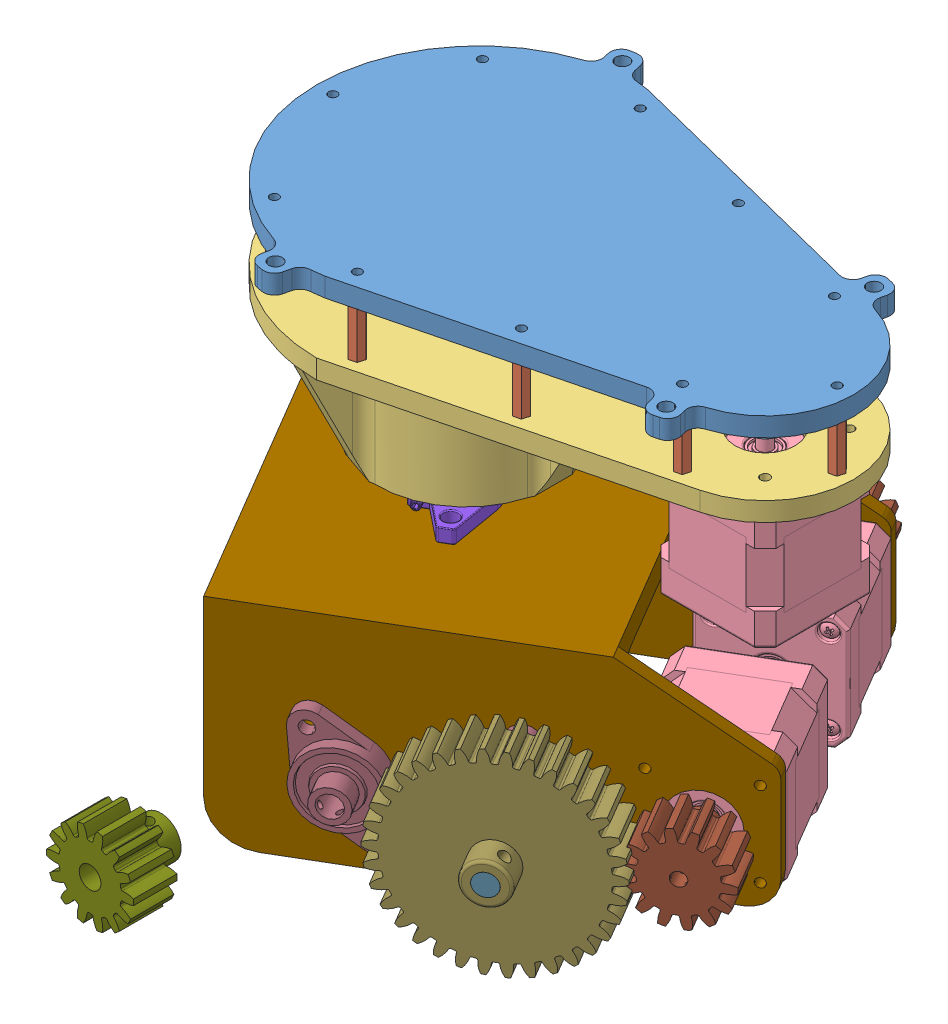
SolidWorks assembly Assembly, configuration Default. Lengths in mm.
Overall size (223.52 202.91 241.25).
33 component instances, 16 part files, 73 mates.
Components (placement in the parent):
- base1-2: base1 [Varsayılan] at (61.0141 100.5381 159.3571) size (197.5 7 137.85)
- tru_dong_20mm-1: tru_dong_20mm [Default] at (-33.0715 80.5381 158.3482) x (-1 0 0) z (0 1 0) size (5.26 5.22 20)
- tru_dong_20mm-2: tru_dong_20mm [Default] at (-16.7501 80.5381 119.6659) x (-1 0 0) z (0 1 0) size (5.26 5.22 20)
- tru_dong_20mm-3: tru_dong_20mm [Default] at (123.4514 80.5381 130.3946) x (-1 0 0) z (0 1 0) size (5.26 5.22 20)
- tru_dong_20mm-4: tru_dong_20mm [Default] at (27.9599 80.5381 210.3868) x (-1 0 0) z (0 1 0) size (5.26 5.22 20)
- tru_dong_20mm-5: tru_dong_20mm [Default] at (76.1904 80.5381 118.4744) x (-1 0 0) z (0 1 0) size (5.26 5.22 20)
- tru_dong_20mm-6: tru_dong_20mm [Default] at (-11.1111 80.5381 201.8162) x (-1 0 0) z (0 1 0) size (5.26 5.22 20)
- tru_dong_20mm-7: tru_dong_20mm [Default] at (152.4285 80.5381 158.3482) x (-1 0 0) z (0 1 0) size (5.26 5.22 20)
- tru_dong_20mm-8: tru_dong_20mm [Default] at (123.4514 80.5381 186.3018) x (-1 0 0) z (0 1 0) size (5.26 5.22 20)
- tru_dong_20mm-9: tru_dong_20mm [Default] at (27.9599 80.5381 106.3096) x (-1 0 0) z (0 1 0) size (5.26 5.22 20)
- tru_dong_20mm-10: tru_dong_20mm [Default] at (76.1904 80.5381 198.222) x (-1 0 0) z (0 1 0) size (5.26 5.22 20)
- base2-1: base2 [Varsayılan] at (55.9285 80.5381 158.3482) x (-1 0 0) z (0 0 1) size (197.5 57 120)
- NEMA 17-1: NEMA 17 [Default] at (121.3113 29.5381 168.7437) x (0 0 1) z (0 1 0) size (42.3 42.3 68)
- GT2_16T-1: GT2_16T [Default] at (125.9285 90.4881 158.3482) x (-0.780314 0 -0.625388) z (0 -1 0) size (13.6 13.6 15.5)
- GT2_80T_8mmSLDPRT-1: GT2_80T_8mmSLDPRT [Default] at (15.9285 83.5381 158.3482) x (0.428158 0 -0.903704) z (0 1 0) size (55 55 18)
- F608ZZ-1: F608ZZ [Défaut] at (15.9285 25.5381 158.3482) x (0.989487 0 0.144619) z (0 -1 0) size (25 25 7)
- SHF-8-1: SHF-8 [Default] at (15.9285 3.5381 158.3482) x (-0.508063 0 -0.86132) z (0.86132 0 -0.508063) size (43 10.01 24)
- base3-1: base3 [Varsayılan] at (15.9285 -5.4619 158.3482) x (0.508063 0 0.86132) z (-0.86132 0 0.508063) size (120 79 155)
- NEMA 17-2: NEMA 17 [Default] at (87.3379 -41.2437 103.4551) x (0.86132 0 -0.508063) z (-0.508063 0 -0.86132) size (42.3 42.3 68)
- NEMA 17-3: NEMA 17 [Default] at (85.5846 -56.2564 130.0315) x (0 -1 0) z (0.508063 0 0.86132) size (42.3 42.3 68)
- truc8_107mm-1: truc8_107mm [Default] at (15.9285 101.5381 158.3482) x (1 0 0) z (0 -1 0) size (8 8 107)
- banh_rang_1-2: banh_rang_1 [Varsayılan] at (123.0936 -45.8609 184.5328) x (-0.491421 0.821267 0.289873) z (-0.508063 0 -0.86132) size (32 32 26)
- banh_rang_1-3: banh_rang_1 [Varsayılan] at (44.8518 -45.8609 51.8896) x (0.859443 -0.065982 -0.506956) z (0.508063 0 0.86132) size (32 32 26)
- banh_rang_2-1: banh_rang_2 [Varsayılan] at (0.9682 -45.8609 71.97) x (0.433616 0.864035 -0.255775) z (0.508063 0 0.86132) size (72 72 26)
- KFL08-1: KFL08 [По умолчанию] at (12.1456 -45.8609 90.9191) x (-0.86132 0 0.508063) z (-0.508063 0 -0.86132) size (27 47.5 16)
- KFL08-2: KFL08 [По умолчанию] at (-29.1978 -45.8609 115.3061) x (-0.745925 -0.5 0.439996) z (-0.508063 0 -0.86132) size (27 47.5 16)
- KFL08-3: KFL08 [По умолчанию] at (73.1132 -45.8609 194.2774) x (0.86132 0 -0.508063) z (0.508063 0 0.86132) size (27 47.5 16)
- KFL08-4: KFL08 [По умолчанию] at (31.7698 -45.8609 218.6645) x (0.745925 0.5 -0.439996) z (0.508063 0 0.86132) size (27 47.5 16)
- banh_rang_2-2: banh_rang_2 [Varsayılan] at (84.2906 -45.8609 213.2265) x (-0.734353 0.522579 0.43317) z (-0.508063 0 -0.86132) size (72 72 26)
- truc8_200mm-1: truc8_200mm [Default] at (-8.177 -45.8609 56.4663) x (0.095955 -0.993775 -0.056601) z (0.508063 0 0.86132) size (8 8 200)
- banh_rang_3-1: banh_rang_3 [Varsayılan] at (-21.551 -45.8609 128.2697) x (0.813523 -0.32849 -0.47987) z (0.508063 0 0.86132) size (72 72 16)
- banh_rang_3-2: banh_rang_3 [Varsayılan] at (1.1002 -45.8609 166.6703) x (0.813523 -0.32849 -0.47987) z (0.508063 0 0.86132) size (72 72 16)
- banh_rang_4-1: banh_rang_4 [Varsayılan] at (-7.9995 -72.1728 264.7065) size (32 32 26)
Mates (geometry in assembly coordinates):
- Coincident1: coincident aligned: plane of tru_dong_20mm-1 through (-33.0715 80.5381 158.3482) normal (0 -1 0); plane of tru_dong_20mm-2 through (-16.7501 80.5381 119.6659) normal (0 -1 0)
- Coincident2: coincident aligned: plane of tru_dong_20mm-2 through (-16.7501 80.5381 119.6659) normal (0 -1 0); plane of tru_dong_20mm-3 through (123.4514 80.5381 130.3946) normal (0 -1 0)
- Coincident3: coincident aligned: plane of tru_dong_20mm-3 through (123.4514 80.5381 130.3946) normal (0 -1 0); plane of tru_dong_20mm-4 through (27.9599 80.5381 210.3868) normal (0 -1 0)
- Coincident4: coincident aligned: plane of tru_dong_20mm-4 through (27.9599 80.5381 210.3868) normal (0 -1 0); plane of tru_dong_20mm-5 through (76.1904 80.5381 118.4744) normal (0 -1 0)
- Coincident5: coincident aligned: plane of tru_dong_20mm-3 through (123.4514 80.5381 130.3946) normal (0 -1 0); plane of tru_dong_20mm-6 through (-11.1111 80.5381 201.8162) normal (0 -1 0)
- Coincident6: coincident aligned: plane of tru_dong_20mm-3 through (123.4514 80.5381 130.3946) normal (0 -1 0); plane of tru_dong_20mm-7 through (152.4285 80.5381 158.3482) normal (0 -1 0)
- Coincident7: coincident aligned: plane of tru_dong_20mm-3 through (123.4514 80.5381 130.3946) normal (0 -1 0); plane of tru_dong_20mm-9 through (27.9599 80.5381 106.3096) normal (0 -1 0)
- Coincident8: coincident aligned: plane of tru_dong_20mm-6 through (-11.1111 80.5381 201.8162) normal (0 -1 0); plane of tru_dong_20mm-8 through (123.4514 80.5381 186.3018) normal (0 -1 0)
- Coincident9: coincident aligned: plane of tru_dong_20mm-8 through (123.4514 80.5381 186.3018) normal (0 -1 0); plane of tru_dong_20mm-10 through (76.1904 80.5381 198.222) normal (0 -1 0)
- Coincident10: coincident anti-aligned: plane of base1-2 through (125.9285 100.5381 158.3482) normal (0 -1 0); plane of tru_dong_20mm-5 through (76.1904 100.5381 118.4744) normal (0 1 0)
- Concentric1: concentric aligned: cylinder of base1-2 through (76.1904 107.5381 118.4744) axis (0 -1 0) radius 1.6; cylinder of tru_dong_20mm-5 through (76.1904 100.5381 118.4744) axis (0 -1 0) radius 1.6
- Concentric2: concentric aligned: cylinder of base1-2 through (-16.7501 107.5381 119.6659) axis (0 -1 0) radius 1.6; cylinder of tru_dong_20mm-2 through (-16.7501 100.5381 119.6659) axis (0 -1 0) radius 1.6
- Concentric3: concentric aligned: cylinder of base1-2 through (-33.0715 107.5381 158.3482) axis (0 -1 0) radius 1.6; cylinder of tru_dong_20mm-1 through (-33.0715 100.5381 158.3482) axis (0 -1 0) radius 1.6
- Concentric4: concentric aligned: cylinder of base1-2 through (27.9599 107.5381 106.3096) axis (0 -1 0) radius 1.6; cylinder of tru_dong_20mm-9 through (27.9599 100.5381 106.3096) axis (0 -1 0) radius 1.6
- Concentric5: concentric aligned: cylinder of base1-2 through (123.4514 107.5381 130.3946) axis (0 -1 0) radius 1.6; cylinder of tru_dong_20mm-3 through (123.4514 100.5381 130.3946) axis (0 -1 0) radius 1.6
- Concentric6: concentric aligned: cylinder of base1-2 through (152.4285 107.5381 158.3482) axis (0 -1 0) radius 1.6; cylinder of tru_dong_20mm-7 through (152.4285 100.5381 158.3482) axis (0 -1 0) radius 1.6
- Coincident11: coincident anti-aligned: circle of base1-2; cylinder of tru_dong_20mm-8 through (123.4514 100.5381 186.3018) axis (0 -1 0) radius 1.6
- Concentric7: concentric aligned: cylinder of base1-2 through (76.1904 107.5381 198.222) axis (0 -1 0) radius 1.6; cylinder of tru_dong_20mm-10 through (76.1904 100.5381 198.222) axis (0 -1 0) radius 1.6
- Concentric8: concentric aligned: cylinder of base1-2 through (27.9599 107.5381 210.3868) axis (0 -1 0) radius 1.6; cylinder of tru_dong_20mm-4 through (27.9599 100.5381 210.3868) axis (0 -1 0) radius 1.6
- Concentric9: concentric aligned: cylinder of base1-2 through (-11.1111 107.5381 201.8162) axis (0 -1 0) radius 1.6; cylinder of tru_dong_20mm-6 through (-11.1111 100.5381 201.8162) axis (0 -1 0) radius 1.6
- Coincident12: coincident: plane of tru_dong_20mm-7 through (152.4285 80.5381 158.3482) normal (0 -1 0); plane of base2-1 through (125.9285 80.5381 158.3482) normal (0 1 0)
- Concentric10: concentric anti-aligned: cylinder of tru_dong_20mm-7 through (152.4285 100.5381 158.3482) axis (0 -1 0) radius 1.6; cylinder of base2-1 through (152.4285 70.5381 158.3482) axis (0 1 0) radius 1.6
- Concentric11: concentric anti-aligned: cylinder of tru_dong_20mm-1 through (-33.0715 100.5381 158.3482) axis (0 -1 0) radius 1.6; cylinder of base2-1 through (-33.0715 70.5381 158.3482) axis (0 1 0) radius 1.6
- Concentric12: concentric aligned: cylinder of base2-1 through (125.9285 80.5381 158.3482) axis (0 -1 0) radius 11; cylinder of NEMA 17-1 through (125.9285 97.5381 158.3482) axis (0 -1 0) radius 2.5
- Coincident13: coincident anti-aligned: plane of base2-1 through (125.9285 73.5381 158.3482) normal (0 -1 0); plane of NEMA 17-1 through (125.9285 73.5381 158.3482) normal (0 1 0)
- Concentric13: concentric anti-aligned: cylinder of base2-1 through (141.4285 80.5381 142.8482) axis (0 -1 0) radius 1.7; cylinder of NEMA 17-1 through (141.4285 69.0381 142.8482) axis (0 1 0) radius 1.5
- Concentric14: concentric aligned: cylinder of NEMA 17-1 through (125.9285 97.5381 158.3482) axis (0 -1 0) radius 2.5; cylinder of GT2_16T-1 through (125.9285 83.1881 158.3482) axis (0 -1 0) radius 2.5
- Coincident14: coincident aligned: plane of NEMA 17-1 through (125.9285 97.5381 158.3482) normal (0 1 0); plane of GT2_16T-1 through (125.9285 97.5381 158.3482) normal (0 1 0)
- Coincident15: coincident aligned: plane of GT2_16T-1 through (125.9285 82.0381 158.3482) normal (0 -1 0); plane of GT2_80T_8mmSLDPRT-1 through (15.9285 82.0381 158.3482) normal (0 -1 0)
- Concentric16: concentric anti-aligned: cylinder of base2-1 through (15.9285 23.5381 158.3482) axis (0 1 0) radius 11; cylinder of GT2_80T_8mmSLDPRT-1 through (15.9285 90.5381 158.3482) axis (0 -1 0) radius 4
- Concentric17: concentric anti-aligned: cylinder of base2-1 through (15.9285 23.5381 158.3482) axis (0 1 0) radius 11; cylinder of F608ZZ-1 through (15.9285 -209.5122 158.3482) axis (0 -1 0) radius 11
- Coincident16: coincident anti-aligned: plane of base2-1 through (15.9285 23.5381 158.3482) normal (0 -1 0); plane of F608ZZ-1 through (15.9285 23.5381 158.3482) normal (0 1 0)
- Concentric18: concentric aligned: cylinder of F608ZZ-1 through (15.9285 -209.5122 158.3482) axis (0 -1 0) radius 4; cylinder of SHF-8-1 through (15.9285 8.5381 158.3482) axis (0 -1 0) radius 4
- Distance1: distance = 10 mm: plane of SHF-8-1 through (15.9285 13.5381 158.3482) normal (0 1 0); plane of base2-1 through (15.9285 23.5381 158.3482) normal (0 -1 0)
- Coincident19: coincident anti-aligned: plane of SHF-8-1 through (15.9285 3.5381 158.3482) normal (0 -1 0); plane of base3-1 through (15.9285 3.5381 158.3482) normal (0 1 0)
- Concentric19: concentric aligned: cylinder of SHF-8-1 through (15.9285 8.5381 158.3482) axis (0 -1 0) radius 4; cylinder of base3-1 through (15.9285 64.5381 158.3482) axis (0 -1 0) radius 7.5
- Concentric20: concentric anti-aligned: cylinder of SHF-8-1 through (24.0575 8.5381 172.1293) axis (0 -1 0) radius 2.75; cylinder of base3-1 through (24.0575 -6.4619 172.1293) axis (0 1 0) radius 3
- Coincident20: coincident anti-aligned: plane of base3-1 through (43.8719 -5.4619 205.7208) normal (-0.508063 0 -0.86132); plane of NEMA 17-3 through (111.9162 -45.8609 165.5838) normal (0.508063 0 0.86132)
- Coincident21: coincident anti-aligned: plane of base3-1 through (-12.015 -5.4619 110.9756) normal (0.508063 0 0.86132); plane of NEMA 17-2 through (56.0292 -45.8609 70.8386) normal (-0.508063 0 -0.86132)
- Concentric21: concentric anti-aligned: cylinder of base3-1 through (56.0292 -45.8609 70.8386) axis (-0.508063 0 -0.86132) radius 11.15; cylinder of NEMA 17-2 through (43.8357 -45.8609 50.167) axis (0.508063 0 0.86132) radius 2.5
- Concentric22: concentric anti-aligned: cylinder of base3-1 through (111.9162 -45.8609 165.5838) axis (0.508063 0 0.86132) radius 11.15; cylinder of NEMA 17-3 through (124.1097 -45.8609 186.2555) axis (-0.508063 0 -0.86132) radius 2.5
- Concentric23: concentric aligned: cylinder of base3-1 through (98.5657 -61.3609 173.4588) axis (0.508063 0 0.86132) radius 1.65; cylinder of NEMA 17-3 through (96.2795 -61.3609 169.5828) axis (0.508063 0 0.86132) radius 1.5
- Concentric24: concentric aligned: cylinder of base3-1 through (42.6788 -61.3609 78.7136) axis (-0.508063 0 -0.86132) radius 1.65; cylinder of NEMA 17-2 through (44.9651 -61.3609 82.5896) axis (-0.508063 0 -0.86132) radius 1.5
- Concentric25: concentric anti-aligned: cylinder of SHF-8-1 through (15.9285 8.5381 158.3482) axis (0 -1 0) radius 4; cylinder of truc8_107mm-1 through (15.9285 -5.4619 158.3482) axis (0 1 0) radius 4
- Coincident23: coincident aligned: plane of base3-1 through (15.9285 -5.4619 158.3482) normal (0 -1 0); plane of truc8_107mm-1 through (15.9285 -5.4619 158.3482) normal (0 -1 0)
- Concentric27: concentric anti-aligned: cylinder of NEMA 17-2 through (43.8357 -45.8609 50.167) axis (0.508063 0 0.86132) radius 2.5; cylinder of banh_rang_1-3 through (53.997 -45.8609 67.3934) axis (-0.508063 0 -0.86132) radius 2.5
- Concentric29: concentric anti-aligned: cylinder of NEMA 17-3 through (124.1097 -45.8609 186.2555) axis (-0.508063 0 -0.86132) radius 2.5; cylinder of banh_rang_1-2 through (113.9485 -45.8609 169.0291) axis (0.508063 0 0.86132) radius 2.5
- Distance5: distance = 2 mm anti-aligned: plane of banh_rang_1-2 through (113.9485 -45.8609 169.0291) normal (-0.508063 0 -0.86132); plane of NEMA 17-3 through (112.9323 -45.8609 167.3064) normal (0.508063 0 0.86132)
- Distance6: distance = 2 mm anti-aligned: plane of banh_rang_1-3 through (53.997 -45.8609 67.3934) normal (0.508063 0 0.86132); plane of NEMA 17-2 through (55.0131 -45.8609 69.116) normal (-0.508063 0 -0.86132)
- Coincident25: coincident anti-aligned: plane of base3-1 through (93.7848 3.5381 182.0839) normal (0.508063 0 0.86132); plane of KFL08-4 through (39.6294 -61.6658 214.0284) normal (-0.508063 0 -0.86132)
- Concentric30: concentric aligned: cylinder of base3-1 through (31.7698 -45.8609 218.6645) axis (-0.508063 0 -0.86132) radius 5; cylinder of KFL08-4 through (34.0561 -45.8609 222.5404) axis (-0.508063 0 -0.86132) radius 4
- Concentric31: concentric aligned: cylinder of base3-1 through (23.9103 -30.0559 223.3006) axis (-0.508063 0 -0.86132) radius 3; cylinder of KFL08-4 through (26.1966 -30.0559 227.1765) axis (-0.508063 0 -0.86132) radius 2.4
- Coincident26: coincident anti-aligned: plane of base3-1 through (93.7848 3.5381 182.0839) normal (0.508063 0 0.86132); plane of KFL08-3 through (73.1132 -64.1109 194.2774) normal (-0.508063 0 -0.86132)
- Concentric32: concentric aligned: cylinder of base3-1 through (73.1132 -45.8609 194.2774) axis (-0.508063 0 -0.86132) radius 5; cylinder of KFL08-3 through (75.3995 -45.8609 198.1534) axis (-0.508063 0 -0.86132) radius 4
- Concentric33: concentric aligned: cylinder of base3-1 through (73.1132 -64.1109 194.2774) axis (-0.508063 0 -0.86132) radius 2.5; cylinder of KFL08-3 through (75.3995 -64.1109 198.1534) axis (-0.508063 0 -0.86132) radius 2.4
- Coincident27: coincident anti-aligned: plane of base3-1 through (32.8172 3.5381 78.7256) normal (-0.508063 0 -0.86132); plane of KFL08-1 through (12.1456 -64.1109 90.9191) normal (0.508063 0 0.86132)
- Coincident29: coincident anti-aligned: plane of base3-1 through (32.8172 3.5381 78.7256) normal (-0.508063 0 -0.86132); plane of KFL08-2 through (-21.3382 -61.6658 110.67) normal (0.508063 0 0.86132)
- Concentric34: concentric anti-aligned: cylinder of base3-1 through (73.1132 -45.8609 194.2774) axis (-0.508063 0 -0.86132) radius 5; cylinder of KFL08-1 through (9.8593 -45.8609 87.0431) axis (0.508063 0 0.86132) radius 4
- Concentric35: concentric anti-aligned: cylinder of base3-1 through (73.1132 -64.1109 194.2774) axis (-0.508063 0 -0.86132) radius 2.5; cylinder of KFL08-1 through (9.8593 -64.1109 87.0431) axis (0.508063 0 0.86132) radius 2.4
- Concentric36: concentric anti-aligned: cylinder of base3-1 through (31.7698 -45.8609 218.6645) axis (-0.508063 0 -0.86132) radius 5; cylinder of KFL08-2 through (-31.4841 -45.8609 111.4302) axis (0.508063 0 0.86132) radius 4
- Concentric37: concentric anti-aligned: cylinder of base3-1 through (23.9103 -30.0559 223.3006) axis (-0.508063 0 -0.86132) radius 3; cylinder of KFL08-2 through (-39.3436 -30.0559 116.0663) axis (0.508063 0 0.86132) radius 2.4
- Concentric39: concentric aligned: cylinder of banh_rang_2-1 through (-22.4027 -45.8609 32.3493) axis (0.508063 0 0.86132) radius 4; cylinder of KFL08-1 through (9.8593 -45.8609 87.0431) axis (0.508063 0 0.86132) radius 4
- GearMate1: gear = 28 : 68 mm: circle of banh_rang_2-1; circle of banh_rang_1-3
- Concentric42: concentric aligned: cylinder of KFL08-3 through (75.3995 -45.8609 198.1534) axis (-0.508063 0 -0.86132) radius 4; cylinder of banh_rang_2-2 through (107.6615 -45.8609 252.8472) axis (-0.508063 0 -0.86132) radius 4
- GearMate2: gear = 68 : 28 mm: circle of banh_rang_1-2; circle of banh_rang_2-2
- Coincident33: coincident aligned: line of banh_rang_1-2 through (137.1086 -34.7912 185.5539) axis (-0.508063 0 -0.86132); line of banh_rang_1-3 through (58.8669 -34.7912 52.9107) axis (-0.508063 0 -0.86132)
- Concentric45: concentric aligned: cylinder of base3-1 through (73.1132 -45.8609 194.2774) axis (-0.508063 0 -0.86132) radius 5; cylinder of truc8_200mm-1 through (93.4357 -45.8609 228.7302) axis (-0.508063 0 -0.86132) radius 4
- Width1: width aligned: plane of base3-1 through (37.3898 -75.4619 86.4774) normal (0.508063 0 0.86132); plane of truc8_200mm-1 through (89.2123 -75.4619 174.332) normal (-0.508063 0 -0.86132); plane of base3-1 through (93.4357 -45.8609 228.7302) normal (0.508063 0 0.86132); plane of truc8_200mm-1 through (-8.177 -45.8609 56.4663) normal (-0.508063 0 -0.86132)
- Concentric46: concentric aligned: cylinder of banh_rang_3-1 through (-25.6155 -45.8609 121.3791) axis (0.508063 0 0.86132) radius 4; cylinder of banh_rang_3-2 through (-2.9643 -45.8609 159.7798) axis (0.508063 0 0.86132) radius 4
- Concentric47: concentric aligned: cylinder of banh_rang_3-1 through (-43.9198 -38.4699 132.1762) axis (0.508063 0 0.86132) radius 2.5; cylinder of banh_rang_3-2 through (-21.2685 -38.4699 170.5768) axis (0.508063 0 0.86132) radius 2.5
- Concentric49: concentric anti-aligned: cylinder of base3-1 through (31.7698 -45.8609 218.6645) axis (-0.508063 0 -0.86132) radius 5; cylinder of banh_rang_3-2 through (-2.9643 -45.8609 159.7798) axis (0.508063 0 0.86132) radius 4
- Coincident34: coincident aligned: plane of banh_rang_2-2 through (93.4357 -45.8609 228.7302) normal (0.508063 0 0.86132); plane of truc8_200mm-1 through (93.4357 -45.8609 228.7302) normal (0.508063 0 0.86132)
- Coincident35: coincident aligned: circle of banh_rang_2-1; plane of truc8_200mm-1 through (-8.177 -45.8609 56.4663) normal (-0.508063 0 -0.86132)
